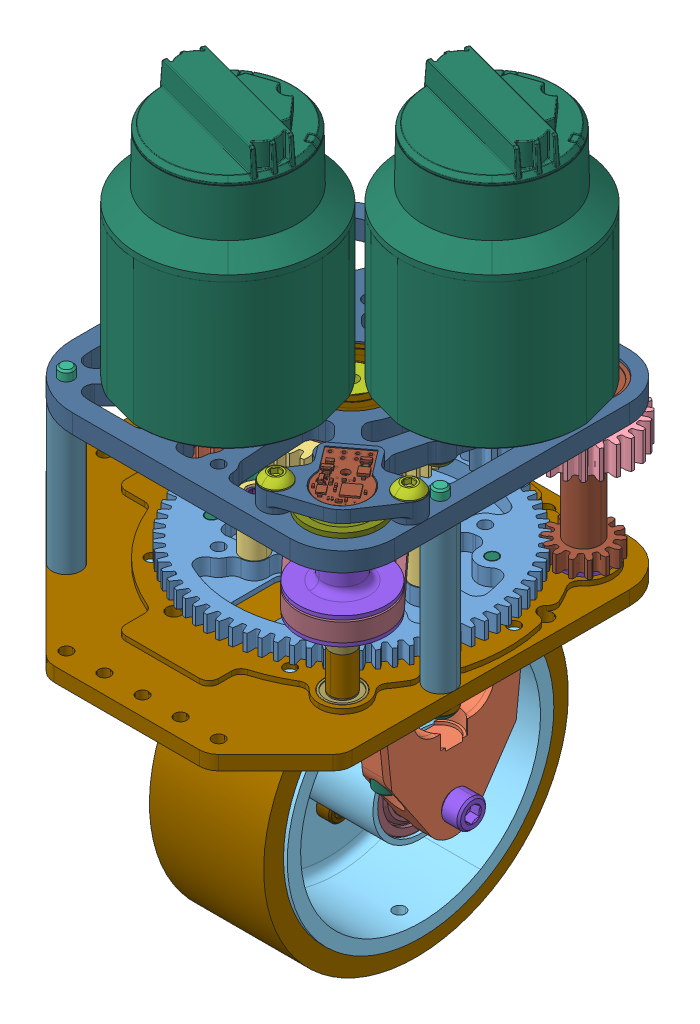
SolidWorks assembly Swerve, configuration Default. Lengths in mm.
Overall size (145.15 256.28 148.25).
84 component instances, 49 part files, 0 mates.
Components (placement in the parent):
- WCP-0360.step-1: WCP-0360.step [Default] at origin size (145.15 256.28 148.25)
  - WCP-0364 Rev1 - WCP X Wheel Module.step-1: WCP-0364 Rev1 - WCP X Wheel Module.step [Default] at (0 -0.825 0) size (95.62 174.54 137.74)
    - WCP-0364-001 Rev1.step-1: WCP-0364-001 Rev1.step [Default] at (0 6.35 0) size (93.93 9.53 93.93)
    - WCP-0366 Rev1_Default_As Machined_.step-1: WCP-0366 Rev1_Default_As Machined_.step [Default] at (-29.2862 -49.2125 0) x (0 0 1) z (-1 0 0) size (51.81 60.46 9.5)
    - WCP-0366 Rev1_Default_As Machined_.step-2: WCP-0366 Rev1_Default_As Machined_.step [Default] at (29.2862 -49.2125 0) x (0 0 -1) z (1 0 0) size (51.81 60.46 9.5)
    - WCP-0364-006 Rev1.step-1: WCP-0364-006 Rev1.step [Default] at (0 -49.2125 0) x (1 0 0) z (0 -0.837962 0.545729) size (56.46 12.67 12.67)
    - WCP-0364-005 Rev2.step-1: WCP-0364-005 Rev2.step [Default] at (-29.2862 -1.2827 0) x (0 -1 0) z (0 0 1) size (54.08 11 11)
    - WCP-0365 Rev2.step-1: WCP-0365 Rev2.step [Default] at (2.3061 -49.2125 0) x (0 -0.866025 -0.5) z (1 0 0) size (88.9 88.9 41.15)
    - WCP-0233 Rev1.step-1: WCP-0233 Rev1.step [Default] at (-18.0375 -49.2125 0) x (0 0 -1) z (0 1 0) size (68.52 16.32 68.56)
    - WCP-0364-002 Rev1.step-1: WCP-0364-002 Rev1.step [Default] at (0 34.5757 0) x (0 -1 0) z (0.999257 0 0.03854) size (51.69 15 15)
    - WCP-0276 Rev1.step-1: WCP-0276 Rev1.step [Default] at (-29.2862 -15.4625 0) x (0 0 1) z (1 0 0) size (25.2 12.86 25.34)
    - WCP-0364-008 Rev1.step-1: WCP-0364-008 Rev1.step [Default] at (2.3061 -49.2125 0) x (1 0 0) z (0 -0.879106 0.476626) size (38.1 101.6 101.6)
    - WCP-0357 Rev1.step-1: WCP-0357 Rev1.step [Default] at origin size (88.91 6.35 88.9)
    - WCP-0784_0375_flanged_thunderhex_bearing.step-1: WCP-0784_0375_flanged_thunderhex_bearing.step [Default] at (-29.2862 12.7 0) x (0 -1 0) z (0.06043 0 0.998172) size (7.11 24.61 24.61)
    - WCP-0775_0_250_radial_bearing.step-1: WCP-0775_0_250_radial_bearing.step [Default] at (-29.2862 -29.3687 0) x (0 -1 0) z (0.460874 0 0.887465) size (4.76 12.7 12.7)
    - WCP-0778_0_500_radial_bearing.step-1: WCP-0778_0_500_radial_bearing.step [Default] at (18.0604 -49.2125 0) x (1 0 0) z (0 -0.205758 0.978603) size (7.94 28.57 28.57)
    - WCP-0778_0_500_radial_bearing.step-2: WCP-0778_0_500_radial_bearing.step [Default] at (-17.8424 -49.2125 0) x (1 0 0) z (0 0.040496 0.99918) size (7.94 28.57 28.57)
    - WCP-0781_0_500_flanged_bearing.step-1: WCP-0781_0_500_flanged_bearing.step [Default] at (0 4.7625 0) x (0.999376 0 -0.035335) z (0.035335 0 0.999376) size (31.12 7.94 31.12)
    - NFS-0018_SHCS_#10-32_1_750L_Default_As Machined_.step-1: NFS-0018_SHCS_#10-32_1_750L_Default_As Machined_.step [Default] at (29.2862 11.1125 17.4625) x (0.988526 0 -0.151053) z (0 1 0) size (7.92 7.92 49.28)
    - NFS-0018_SHCS_#10-32_1_750L_Default_As Machined_.step-2: NFS-0018_SHCS_#10-32_1_750L_Default_As Machined_.step [Default] at (29.2862 11.1125 -17.4625) x (0.988526 0 -0.151053) z (0 1 0) size (7.92 7.92 49.28)
    - NFS-0018_SHCS_#10-32_1_750L_Default_As Machined_.step-3: NFS-0018_SHCS_#10-32_1_750L_Default_As Machined_.step [Default] at (-29.2862 11.1125 17.4625) x (0.988526 0 -0.151053) z (0 1 0) size (7.92 7.92 49.28)
    - NFS-0018_SHCS_#10-32_1_750L_Default_As Machined_.step-4: NFS-0018_SHCS_#10-32_1_750L_Default_As Machined_.step [Default] at (-29.2862 11.1125 -17.4625) x (0.988526 0 -0.151053) z (0 1 0) size (7.92 7.92 49.28)
    - 8-32 BHCS_0.500.step-1: 8-32 BHCS_0.500.step [Default] at (-29.2862 23.8633 0) x (0.940105 0 -0.340884) z (0.340884 0 0.940105) size (7.92 14.92 7.92)
    - NFS-0059_SHCS_#4-40_0_875L_91251A113.step-1: NFS-0059_SHCS_#4-40_0_875L_91251A113.step [Default] at (23.876 3.0654 0) x (0.520663 0 0.853762) z (0 -1 0) size (4.65 4.65 25.08)
    - NFS-0059_SHCS_#4-40_0_875L_91251A113.step-2: NFS-0059_SHCS_#4-40_0_875L_91251A113.step [Default] at (-11.938 3.0654 -20.6772) x (0.520663 0 0.853762) z (0 -1 0) size (4.65 4.65 25.08)
    - NFS-0059_SHCS_#4-40_0_875L_91251A113.step-3: NFS-0059_SHCS_#4-40_0_875L_91251A113.step [Default] at (-11.938 3.0654 20.6772) x (0.520663 0 0.853762) z (0 -1 0) size (4.65 4.65 25.08)
    - 10-32 SHCS - No Thread_WCP-0265 - 0.375.step-1: 10-32 SHCS - No Thread_WCP-0265 - 0.375.step [Default] at (-8.2862 -69.85 0) x (0 0.591573 -0.806252) z (0 -0.806252 -0.591573) size (7.67 14.35 7.67)
    - 10-32 SHCS - No Thread_WCP-0265 - 0.375.step-2: 10-32 SHCS - No Thread_WCP-0265 - 0.375.step [Default] at (-8.2862 -38.8937 17.8726) x (0 -0.796051 -0.60523) z (0 -0.60523 0.796051) size (7.67 14.35 7.67)
    - 10-32 SHCS - No Thread_WCP-0265 - 0.375.step-3: 10-32 SHCS - No Thread_WCP-0265 - 0.375.step [Default] at (-8.2862 -59.5312 17.8726) x (0 -0.796051 -0.60523) z (0 -0.60523 0.796051) size (7.67 14.35 7.67)
    - 10-32 SHCS - No Thread_WCP-0265 - 0.375.step-4: 10-32 SHCS - No Thread_WCP-0265 - 0.375.step [Default] at (-8.2862 -59.5312 -17.8726) x (0 -0.796051 -0.60523) z (0 -0.60523 0.796051) size (7.67 14.35 7.67)
    - 10-32 SHCS - No Thread_WCP-0265 - 0.375.step-5: 10-32 SHCS - No Thread_WCP-0265 - 0.375.step [Default] at (-8.2862 -38.8937 -17.8726) x (0 -0.796051 -0.60523) z (0 -0.60523 0.796051) size (7.67 14.35 7.67)
    - 10-32 SHCS - No Thread_WCP-0265 - 0.375.step-6: 10-32 SHCS - No Thread_WCP-0265 - 0.375.step [Default] at (-8.2862 -28.575 0) x (0 -0.796051 -0.60523) z (0 -0.60523 0.796051) size (7.67 14.35 7.67)
    - NFS-0024_250-20_thin_locknut_90566A029.step-1: NFS-0024_250-20_thin_locknut_90566A029.step [Default] at (-34.0362 -49.2125 0) x (0 0.824738 0.565516) z (0 -0.565516 0.824738) size (11.14 5.19 12.86)
    - WCP-0229 Rev1.step-1: WCP-0229 Rev1.step [Default] at (-22.6822 -49.2125 0) size (0.89 16.1 14.34)
    - WCP-0229 Rev1.step-2: WCP-0229 Rev1.step [Default] at (22.6822 -49.2125 0) size (0.89 16.1 14.34)
    - WCP-0367-002 Rev3.step-1: WCP-0367-002 Rev3.step [Default] at (0 28.6559 0) x (0 0 -1) z (1 0 0) size (49.74 26.04 44.2)
    - WCP-0367-006 Rev1.step-1: WCP-0367-006 Rev1.step [Default] at (-29.2862 -3.81 0) size (17.27 17.14 17.27)
    - WCP-0367-010 Rev1.step-1: WCP-0367-010 Rev1.step [Default] at (-29.2862 22.2758 0) x (0 0 1) z (-1 0 0) size (12.7 4.76 12.7)
    - WCP-0434 Rev1.step-1: WCP-0434 Rev1.step [Default] at (-29.2862 19 0) x (-0.327758 0 -0.944762) z (0 -1 0) size (30.3 30.48 12.6)
    - 217-5464_24T_500_hex_steel.step-1: 217-5464_24T_500_hex_steel.step [Default] at (0 19 0) x (0.428371 0 0.903603) z (0 -1 0) size (32.87 32.87 12.6)
    - NFS-0059_SHCS_#4-40_0_875L_91251A113.step-4: NFS-0059_SHCS_#4-40_0_875L_91251A113.step [Default] at (23.876 4.3561 0) x (0.431119 0 0.902295) z (0 -1 0) size (4.65 4.65 25.08)
    - NFS-0059_SHCS_#4-40_0_875L_91251A113.step-5: NFS-0059_SHCS_#4-40_0_875L_91251A113.step [Default] at (-11.938 4.3561 -20.6772) x (0.431119 0 0.902295) z (0 -1 0) size (4.65 4.65 25.08)
    - 0250-20_3L_SHCS_91251A554.step-1: 0250-20_3L_SHCS_91251A554.step [Default] at (-0.8888 -49.2125 0) x (0 -0.133483 -0.991051) z (1 0 0) size (9.53 9.53 82.55)
  - WCP-0360-001 Rev1.step-1: WCP-0360-001 Rev1.step [Default] at origin size (133.35 8 133.35)
  - WCP-0360-002 Rev2.step-1: WCP-0360-002 Rev2.step [Default] at (0 53.1812 0) size (111.12 6.35 111.12)
  - WCP-0364-003 Rev1.step-1: WCP-0364-003 Rev1.step [Default] at (38.669 7.5147 -38.669) x (0.999625 0 -0.027384) z (0 1 0) size (20.01 20.32 56.54)
  - WCP-0364-004 Rev1.step-1: WCP-0364-004 Rev1.step [Default] at (36.5633 23.984 39.7383) x (0 1 0) z (-0.749459 0 0.66205) size (58.72 11 11)
  - WCP-0367-009 Rev1.step-1: WCP-0367-009 Rev1.step [Default] at (0 49.7563 0) size (38.1 0.5 38.1)
  - WCP-0387 Rev1.step-1: WCP-0387 Rev1.step [Default] at (49.2125 26.1937 19.7361) x (0 -1 0) z (0.990981 0 -0.134001) size (47.62 9.5 9.5)
  - WCP-0387 Rev1.step-2: WCP-0387 Rev1.step [Default] at (-47.625 26.1937 47.625) x (0 -1 0) z (0.879738 0 -0.475459) size (47.62 9.5 9.5)
  - WCP-0387 Rev1.step-3: WCP-0387 Rev1.step [Default] at (-19.7361 26.1937 -49.2125) x (0 -1 0) z (0.990981 0 -0.134001) size (47.62 9.5 9.5)
  - 217-6515_Falcon_500_Falcon Medium Shaft_As Machined_.step-1: 217-6515_Falcon_500_Falcon Medium Shaft_As Machined_.step [Default] at (23.3487 82.5562 -23.3487) x (-0.707107 0 0.707107) z (0 -1 0) size (60 60 104.7)
  - 217-6515_Falcon_500_Falcon Medium Shaft_As Machined_.step-2: 217-6515_Falcon_500_Falcon Medium Shaft_As Machined_.step [Default] at (-20.7085 82.5562 20.7085) x (-0.707107 0 0.707107) z (0 -1 0) size (60 60 104.7)
  - WCP-0779_0_375_flanged_bearing.step-1: WCP-0779_0_375_flanged_bearing.step [Default] at (36.5633 57.9438 39.7383) x (0 -1 0) z (0.994003 0 0.109352) size (7.11 24.61 24.61)
  - WCP-0775_0_250_radial_bearing.step-1: WCP-0775_0_250_radial_bearing.step [Default] at (36.5633 1.6187 39.7383) x (0 1 0) z (-0.219544 0 0.975603) size (4.76 12.7 12.7)
  - WCP-0041_0_250_radial_bearing.step-1: WCP-0041_0_250_radial_bearing.step [Default] at (38.669 1.5108 -38.669) x (-0.292072 0 0.956396) z (0 -1 0) size (15.88 15.88 4.98)
  - WCP-0784_0375_flanged_thunderhex_bearing.step-1: WCP-0784_0375_flanged_thunderhex_bearing.step [Default] at (38.669 48.4188 -38.669) x (0 1 0) z (0.455959 0 0.890001) size (7.11 24.61 24.61)
  - WCP-0785_0_500_flanged_thunderhex_bearing.step-1: WCP-0785_0_500_flanged_thunderhex_bearing.step [Default] at (0 51.8875 0) x (1 0 0) z (0 -1 0) size (31.12 31.12 7.94)
  - 217-6915_Falcon_8T.step-1: 217-6915_Falcon_8T.step [Default] at (23.3487 42.1912 -23.3487) x (0.394772 0 -0.918779) z (0 1 0) size (13.62 13.62 19.06)
  - 217-6919_Falcon_12T.step-1: 217-6919_Falcon_12T.step [Default] at (-20.7085 42.1912 20.7085) x (-0.353628 0 -0.935386) z (0 1 0) size (17.78 17.78 19.05)
  - WCP-0542 Rev1.step-1: WCP-0542 Rev1.step [Default] at (0 41.5942 0) x (0.777907 0 0.628379) z (0 -1 0) size (45.61 45.72 12.65)
  - WCP-0538 Rev1.step-1: WCP-0538 Rev1.step [Default] at (38.669 42.0941 -38.669) x (0.789433 0 0.613837) z (0 -1 0) size (32.86 32.86 12.65)
  - 10-32 BHCS - No Thread_WCP-0251 - 0.250.step-1: 10-32 BHCS - No Thread_WCP-0251 - 0.250.step [Default] at (-33.4155 -4 33.4155) x (-0.592653 0 -0.805458) z (-0.805458 0 0.592653) size (9.17 8.92 9.17)
  - 10-32 BHCS - No Thread_WCP-0261 - 2.500.step-1: 10-32 BHCS - No Thread_WCP-0261 - 2.500.step [Default] at (-47.625 -4 47.625) x (0.091149 0 -0.995837) z (-0.995837 0 -0.091149) size (9.17 66.07 9.17)
  - 10-32 BHCS - No Thread_WCP-0261 - 2.500.step-2: 10-32 BHCS - No Thread_WCP-0261 - 2.500.step [Default] at (49.2125 -4 19.7361) x (-0.602957 0 -0.797773) z (-0.797773 0 0.602957) size (9.17 66.07 9.17)
  - 10-32 BHCS - No Thread_WCP-0261 - 2.500.step-3: 10-32 BHCS - No Thread_WCP-0261 - 2.500.step [Default] at (-19.7361 -4 -49.2125) x (-0.592653 0 -0.805458) z (-0.805458 0 0.592653) size (9.17 66.07 9.17)
  - 10-32 BHCS - No Thread_WCP-0253 - 0.500.step-1: 10-32 BHCS - No Thread_WCP-0253 - 0.500.step [Default] at (49.2125 62.9348 30.146) x (0.998872 0 0.047489) z (-0.047489 0 0.998872) size (9.17 15.27 9.17)
  - 10-32 BHCS - No Thread_WCP-0253 - 0.500.step-2: 10-32 BHCS - No Thread_WCP-0253 - 0.500.step [Default] at (23.914 62.9348 49.3306) x (0.998872 0 0.047489) z (-0.047489 0 0.998872) size (9.17 15.27 9.17)
  - 10-32 BHCS - No Thread_WCP-0253 - 0.500.step-3: 10-32 BHCS - No Thread_WCP-0253 - 0.500.step [Default] at (29.9227 50.0063 1.1859) x (-0.690184 0 0.723634) z (0.723634 0 0.690184) size (9.17 15.27 9.17)
  - 10-32 BHCS - No Thread_WCP-0253 - 0.500.step-4: 10-32 BHCS - No Thread_WCP-0253 - 0.500.step [Default] at (16.7747 50.0063 -47.8832) x (-0.690184 0 0.723634) z (0.723634 0 0.690184) size (9.17 15.27 9.17)
  - 10-32 BHCS - No Thread_WCP-0253 - 0.500.step-5: 10-32 BHCS - No Thread_WCP-0253 - 0.500.step [Default] at (-14.1345 50.0063 45.243) x (-0.690184 0 0.723634) z (0.723634 0 0.690184) size (9.17 15.27 9.17)
  - 10-32 BHCS - No Thread_WCP-0253 - 0.500.step-6: 10-32 BHCS - No Thread_WCP-0253 - 0.500.step [Default] at (-27.2825 50.0063 -3.826) x (-0.690184 0 0.723634) z (0.723634 0 0.690184) size (9.17 15.27 9.17)
  - 8-32 BHCS_0.500.step-1: 8-32 BHCS_0.500.step [Default] at (-20.7085 32.6662 20.7085) x (0.226967 0 -0.973902) z (-0.973902 0 -0.226967) size (7.92 14.92 7.92)
  - 8-32 BHCS_0.500.step-2: 8-32 BHCS_0.500.step [Default] at (23.3487 32.6662 -23.3487) x (0.226967 0 -0.973902) z (-0.973902 0 -0.226967) size (7.92 14.92 7.92)
  - WCP-0367-003 Rev2.step-1: WCP-0367-003 Rev2.step [Default] at (36.5633 25.8309 39.7383) x (0.279734 0 -0.960077) z (0 -1 0) size (29.05 29.05 26.83)
  - WCP-0367-004 Rev1.step-1: WCP-0367-004 Rev1.step [Default] at (36.5633 10.4711 39.7383) size (8 12.7 8)
  - WCP-0367-012 Rev1_Straight.step-1: WCP-0367-012 Rev1_Straight.step [Default] at (36.5633 60.9155 39.7383) x (-0.796803 0 0.604239) z (-0.604239 0 -0.796803) size (41.27 6.58 26.97)
  - CANcoder.step-1: CANcoder.step [Default] at (36.5633 59.1546 39.7383) x (-0.796803 0 0.604239) z (0 1 0) size (15.94 23.28 4.54)
  - WCP-0156 Rev1.step-1: WCP-0156 Rev1.step [Default] at (36.5633 51.5938 39.7383) size (6.35 12.7 6.35)
  - Encoder Belt.step-1: Encoder Belt.step [Default] at (18.2816 30.8309 19.8691) x (0.677097 0 0.735894) z (-0.735894 0 0.677097) size (83.28 6 29.28)
  - 10-32 BHCS - No Thread_WCP-0251 - 0.250.step-2: 10-32 BHCS - No Thread_WCP-0251 - 0.250.step [Default] at (-42.106 -4 -21.4541) x (0.582896 0 -0.812547) z (-0.812547 0 -0.582896) size (9.17 8.92 9.17)
  - 10-32 BHCS - No Thread_WCP-0251 - 0.250.step-3: 10-32 BHCS - No Thread_WCP-0251 - 0.250.step [Default] at (7.3926 -4 -46.6749) x (0.952903 0 0.303276) z (0.303276 0 -0.952903) size (9.17 8.92 9.17)
  - 10-32 BHCS - No Thread_WCP-0251 - 0.250.step-4: 10-32 BHCS - No Thread_WCP-0251 - 0.250.step [Default] at (46.6749 -4 -7.3926) x (0.00603 0 0.999982) z (0.999982 0 -0.00603) size (9.17 8.92 9.17)
  - 10-32 BHCS - No Thread_WCP-0251 - 0.250.step-5: 10-32 BHCS - No Thread_WCP-0251 - 0.250.step [Default] at (21.4541 -4 42.106) x (-0.949176 0 0.314746) z (0.314746 0 0.949176) size (9.17 8.92 9.17)
